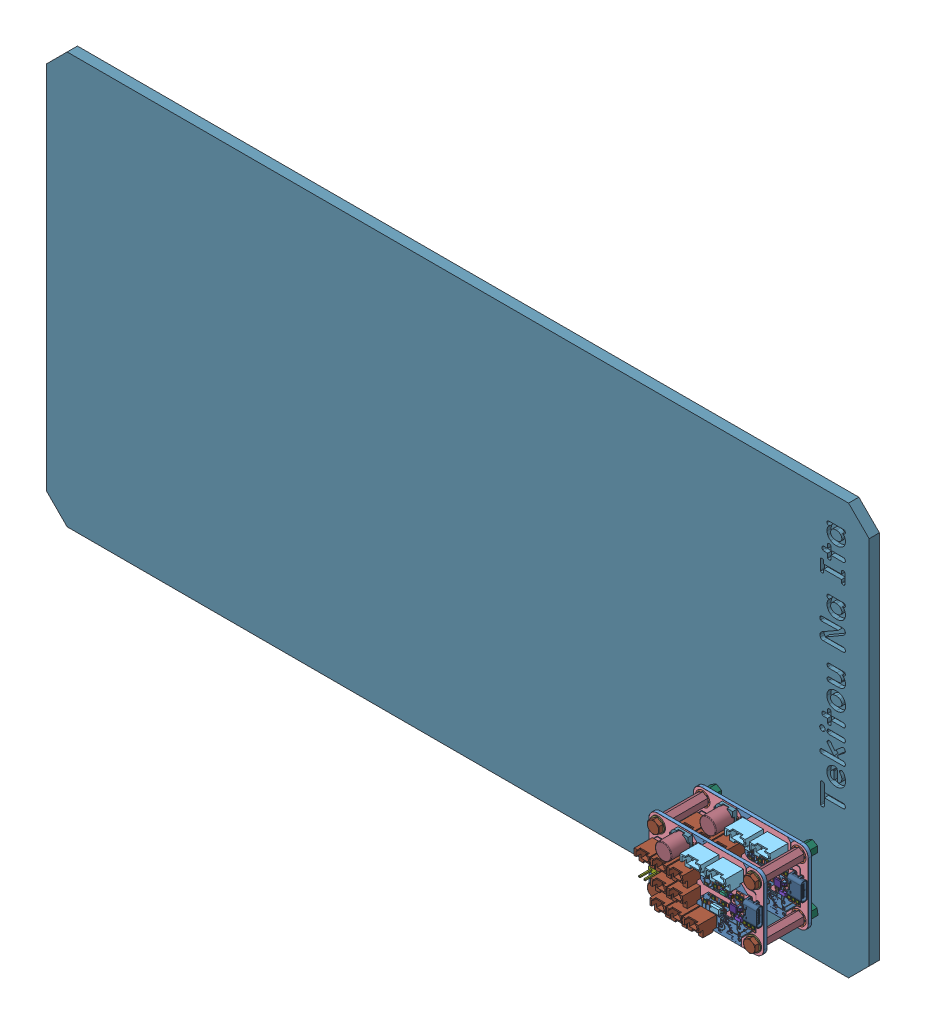
SolidWorks assembly USB_JST-XH_Converter組立サンプル図, configuration ﾃﾞﾌｫﾙﾄ. Lengths in mm.
Overall size (400 200 53.63).
364 component instances, 69 part files, 31 mates.
Components (placement in the parent):
- Board_Geoms_f1fe-1: Board_Geoms_f1fe [ﾃﾞﾌｫﾙﾄ] at (-33.7897 -17.3903 -15.0698) size (55.86 35.85 1.7)
  - Pcb_f1fe-1: Pcb_f1fe [ﾃﾞﾌｫﾙﾄ] at origin size (55.86 35.85 1.6)
  - topPads_f1fe_1-1: topPads_f1fe_1 [ﾃﾞﾌｫﾙﾄ] at (0 0 0.02) size (53.76 33.72 0)
  - topTracks_f1fe-1: topTracks_f1fe [ﾃﾞﾌｫﾙﾄ] at (0 0 0.01) size (44.55 27.82 0)
  - topZones_f1fe-1: topZones_f1fe [ﾃﾞﾌｫﾙﾄ] at (0 0 0.01) size (55.73 35.75 0)
  - botPads_f1fe-1: botPads_f1fe [ﾃﾞﾌｫﾙﾄ] at (0 0 -1.62) size (53.76 33.72 0)
  - botTracks_f1fe-1: botTracks_f1fe [ﾃﾞﾌｫﾙﾄ] at (0 0 -1.61) size (22.1 13.27 0)
  - botZones_f1fe-1: botZones_f1fe [ﾃﾞﾌｫﾙﾄ] at (0 0 -1.61) size (55.76 35.75 0)
  - bottopSilks_f115-1: bottopSilks_f115 [ﾃﾞﾌｫﾙﾄ] at origin size (54.02 34.57 0.01)
  - botSilks_30d3-1: botSilks_30d3 [ﾃﾞﾌｫﾙﾄ] at (0 0 -1.67) size (46.62 31.58 0.02)
- Step_Models_f1fe-1: Step_Models_f1fe [ﾃﾞﾌｫﾙﾄ] at (-33.7897 -17.3903 -15.0698) size (53.92 34.35 13.46)
  - Top_f1fe_1-1: Top_f1fe_1 [ﾃﾞﾌｫﾙﾄ] at origin size (53.92 34.35 13.46)
    - USB1_CUI_DEVICES_UJC-HP-3-SMT-TR_639B4C46-1: USB1_CUI_DEVICES_UJC-HP-3-SMT-TR_639B4C46 [ﾃﾞﾌｫﾙﾄ] at (171.8711 -104.4286 1.3) x (0 1 0) z (1 0 0) size (8.95 4.27 6.9)
    - PORT1_B02B-XASK-1_639C336B-1: PORT1_B02B-XASK-1_639C336B [ﾃﾞﾌｫﾙﾄ] at (125.984 -101.854 0) x (1 0 0) z (0 -1 0) size (7.5 12.2 6.4)
    - PORT1_B02B-XASK-1_639C336B-2: PORT1_B02B-XASK-1_639C336B [ﾃﾞﾌｫﾙﾄ] at (133.9611 -101.854 0) x (1 0 0) z (0 -1 0) size (7.5 12.2 6.4)
    - PORT1_B02B-XASK-1_639C336B-3: PORT1_B02B-XASK-1_639C336B [ﾃﾞﾌｫﾙﾄ] at (141.986 -101.854 0) x (1 0 0) z (0 -1 0) size (7.5 12.2 6.4)
    - PORT1_B02B-XASK-1_639C336B-4: PORT1_B02B-XASK-1_639C336B [ﾃﾞﾌｫﾙﾄ] at (133.9711 -110.4186 0) x (1 0 0) z (0 -1 0) size (7.5 12.2 6.4)
    - PORT1_B02B-XASK-1_639C336B-5: PORT1_B02B-XASK-1_639C336B [ﾃﾞﾌｫﾙﾄ] at (141.9611 -110.4486 0) x (1 0 0) z (0 -1 0) size (7.5 12.2 6.4)
    - SW2_SMLE1_639B495B-1: SW2_SMLE1_639B495B [ﾃﾞﾌｫﾙﾄ] at (148.5711 -101.9286 0) x (-1 0 0) z (0 1 0) size (1.6 0.36 0.8)
    - R2_RT1220P-101-M004_639B496B-1: R2_RT1220P-101-M004_639B496B [ﾃﾞﾌｫﾙﾄ] at (149.3711 -96.9286 0) x (1 0 0) z (0 -1 0) size (2 0.5 1.25)
      - RT1220P-101-M-1: RT1220P-101-M [ﾃﾞﾌｫﾙﾄ] at origin size (0.4 0.5 1.25)
      - RT1220P-101-M001-1: RT1220P-101-M001 [ﾃﾞﾌｫﾙﾄ] at origin size (0.4 0.5 1.25)
      - RT1220P-101-M002-1: RT1220P-101-M002 [ﾃﾞﾌｫﾙﾄ] at origin size (1.95 0.45 1.25)
      - RT1220P-101-M003-1: RT1220P-101-M003 [ﾃﾞﾌｫﾙﾄ] at origin size (1.2 0.03 1.25)
    - R2_RT1220P-101-M004_639B496B-2: R2_RT1220P-101-M004_639B496B [ﾃﾞﾌｫﾙﾄ] at (164.0711 -102.6286 0) x (0 1 0) z (1 0 0) size (2 0.5 1.25)
      - RT1220P-101-M-1: RT1220P-101-M [ﾃﾞﾌｫﾙﾄ] at origin size (0.4 0.5 1.25)
      - RT1220P-101-M001-1: RT1220P-101-M001 [ﾃﾞﾌｫﾙﾄ] at origin size (0.4 0.5 1.25)
      - RT1220P-101-M002-1: RT1220P-101-M002 [ﾃﾞﾌｫﾙﾄ] at origin size (1.95 0.45 1.25)
      - RT1220P-101-M003-1: RT1220P-101-M003 [ﾃﾞﾌｫﾙﾄ] at origin size (1.2 0.03 1.25)
    - R2_RT1220P-101-M004_639B496B-3: R2_RT1220P-101-M004_639B496B [ﾃﾞﾌｫﾙﾄ] at (166.0711 -102.6286 0) x (0 1 0) z (1 0 0) size (2 0.5 1.25)
      - RT1220P-101-M-1: RT1220P-101-M [ﾃﾞﾌｫﾙﾄ] at origin size (0.4 0.5 1.25)
      - RT1220P-101-M001-1: RT1220P-101-M001 [ﾃﾞﾌｫﾙﾄ] at origin size (0.4 0.5 1.25)
      - RT1220P-101-M002-1: RT1220P-101-M002 [ﾃﾞﾌｫﾙﾄ] at origin size (1.95 0.45 1.25)
      - RT1220P-101-M003-1: RT1220P-101-M003 [ﾃﾞﾌｫﾙﾄ] at origin size (1.2 0.03 1.25)
    - PORT1_B02B-XASK-1_639C336B-6: PORT1_B02B-XASK-1_639C336B [ﾃﾞﾌｫﾙﾄ] at (133.5711 -118.9286 0) x (1 0 0) z (0 -1 0) size (7.5 12.2 6.4)
    - PORT1_B02B-XASK-1_639C336B-7: PORT1_B02B-XASK-1_639C336B [ﾃﾞﾌｫﾙﾄ] at (141.5711 -118.9286 0) x (1 0 0) z (0 -1 0) size (7.5 12.2 6.4)
    - PORT1_B02B-XASK-1_639C336B-8: PORT1_B02B-XASK-1_639C336B [ﾃﾞﾌｫﾙﾄ] at (149.5711 -118.9286 0) x (1 0 0) z (0 -1 0) size (7.5 12.2 6.4)
    - C1_CAP_GCM21B_MUR003_639B4A01-1: C1_CAP_GCM21B_MUR003_639B4A01 [ﾃﾞﾌｫﾙﾄ] at (161.0711 -103.4286 0) size (2.01 1.24 1.25)
      - CAP_GCM21B_MUR-1: CAP_GCM21B_MUR [ﾃﾞﾌｫﾙﾄ] at origin size (1.09 1.21 1.21)
      - CAP_GCM21B_MUR001-1: CAP_GCM21B_MUR001 [ﾃﾞﾌｫﾙﾄ] at origin size (0.46 1.24 1.25)
      - CAP_GCM21B_MUR002-1: CAP_GCM21B_MUR002 [ﾃﾞﾌｫﾙﾄ] at origin size (0.46 1.24 1.25)
    - C1_CAP_GCM21B_MUR003_639B4A01-2: C1_CAP_GCM21B_MUR003_639B4A01 [ﾃﾞﾌｫﾙﾄ] at (165.5711 -106.9286 0) x (0 -1 0) z (0 0 1) size (2.01 1.24 1.25)
      - CAP_GCM21B_MUR-1: CAP_GCM21B_MUR [ﾃﾞﾌｫﾙﾄ] at origin size (1.09 1.21 1.21)
      - CAP_GCM21B_MUR001-1: CAP_GCM21B_MUR001 [ﾃﾞﾌｫﾙﾄ] at origin size (0.46 1.24 1.25)
      - CAP_GCM21B_MUR002-1: CAP_GCM21B_MUR002 [ﾃﾞﾌｫﾙﾄ] at origin size (0.46 1.24 1.25)
    - R2_RT1220P-101-M004_639B496B-4: R2_RT1220P-101-M004_639B496B [ﾃﾞﾌｫﾙﾄ] at (171.5711 -111.6286 0) x (0 1 0) z (1 0 0) size (2 0.5 1.25)
      - RT1220P-101-M-1: RT1220P-101-M [ﾃﾞﾌｫﾙﾄ] at origin size (0.4 0.5 1.25)
      - RT1220P-101-M001-1: RT1220P-101-M001 [ﾃﾞﾌｫﾙﾄ] at origin size (0.4 0.5 1.25)
      - RT1220P-101-M002-1: RT1220P-101-M002 [ﾃﾞﾌｫﾙﾄ] at origin size (1.95 0.45 1.25)
      - RT1220P-101-M003-1: RT1220P-101-M003 [ﾃﾞﾌｫﾙﾄ] at origin size (1.2 0.03 1.25)
    - R2_RT1220P-101-M004_639B496B-5: R2_RT1220P-101-M004_639B496B [ﾃﾞﾌｫﾙﾄ] at (167.5711 -111.6286 0) x (0 1 0) z (1 0 0) size (2 0.5 1.25)
      - RT1220P-101-M-1: RT1220P-101-M [ﾃﾞﾌｫﾙﾄ] at origin size (0.4 0.5 1.25)
      - RT1220P-101-M001-1: RT1220P-101-M001 [ﾃﾞﾌｫﾙﾄ] at origin size (0.4 0.5 1.25)
      - RT1220P-101-M002-1: RT1220P-101-M002 [ﾃﾞﾌｫﾙﾄ] at origin size (1.95 0.45 1.25)
      - RT1220P-101-M003-1: RT1220P-101-M003 [ﾃﾞﾌｫﾙﾄ] at origin size (1.2 0.03 1.25)
    - R2_RT1220P-101-M004_639B496B-6: R2_RT1220P-101-M004_639B496B [ﾃﾞﾌｫﾙﾄ] at (153.5711 -100.2286 0) x (0 -1 0) z (-1 0 0) size (2 0.5 1.25)
      - RT1220P-101-M-1: RT1220P-101-M [ﾃﾞﾌｫﾙﾄ] at origin size (0.4 0.5 1.25)
      - RT1220P-101-M001-1: RT1220P-101-M001 [ﾃﾞﾌｫﾙﾄ] at origin size (0.4 0.5 1.25)
      - RT1220P-101-M002-1: RT1220P-101-M002 [ﾃﾞﾌｫﾙﾄ] at origin size (1.95 0.45 1.25)
      - RT1220P-101-M003-1: RT1220P-101-M003 [ﾃﾞﾌｫﾙﾄ] at origin size (1.2 0.03 1.25)
    - R2_RT1220P-101-M004_639B496B-7: R2_RT1220P-101-M004_639B496B [ﾃﾞﾌｫﾙﾄ] at (154.8711 -96.7286 0) x (1 0 0) z (0 -1 0) size (2 0.5 1.25)
      - RT1220P-101-M-1: RT1220P-101-M [ﾃﾞﾌｫﾙﾄ] at origin size (0.4 0.5 1.25)
      - RT1220P-101-M001-1: RT1220P-101-M001 [ﾃﾞﾌｫﾙﾄ] at origin size (0.4 0.5 1.25)
      - RT1220P-101-M002-1: RT1220P-101-M002 [ﾃﾞﾌｫﾙﾄ] at origin size (1.95 0.45 1.25)
      - RT1220P-101-M003-1: RT1220P-101-M003 [ﾃﾞﾌｫﾙﾄ] at origin size (1.2 0.03 1.25)
    - R2_RT1220P-101-M004_639B496B-8: R2_RT1220P-101-M004_639B496B [ﾃﾞﾌｫﾙﾄ] at (156.8711 -101.4286 0) x (1 0 0) z (0 -1 0) size (2 0.5 1.25)
      - RT1220P-101-M-1: RT1220P-101-M [ﾃﾞﾌｫﾙﾄ] at origin size (0.4 0.5 1.25)
      - RT1220P-101-M001-1: RT1220P-101-M001 [ﾃﾞﾌｫﾙﾄ] at origin size (0.4 0.5 1.25)
      - RT1220P-101-M002-1: RT1220P-101-M002 [ﾃﾞﾌｫﾙﾄ] at origin size (1.95 0.45 1.25)
      - RT1220P-101-M003-1: RT1220P-101-M003 [ﾃﾞﾌｫﾙﾄ] at origin size (1.2 0.03 1.25)
    - R2_RT1220P-101-M004_639B496B-9: R2_RT1220P-101-M004_639B496B [ﾃﾞﾌｫﾙﾄ] at (153.2711 -103.4286 0) x (-1 0 0) z (0 1 0) size (2 0.5 1.25)
      - RT1220P-101-M-1: RT1220P-101-M [ﾃﾞﾌｫﾙﾄ] at origin size (0.4 0.5 1.25)
      - RT1220P-101-M001-1: RT1220P-101-M001 [ﾃﾞﾌｫﾙﾄ] at origin size (0.4 0.5 1.25)
      - RT1220P-101-M002-1: RT1220P-101-M002 [ﾃﾞﾌｫﾙﾄ] at origin size (1.95 0.45 1.25)
      - RT1220P-101-M003-1: RT1220P-101-M003 [ﾃﾞﾌｫﾙﾄ] at origin size (1.2 0.03 1.25)
    - R2_RT1220P-101-M004_639B496B-10: R2_RT1220P-101-M004_639B496B [ﾃﾞﾌｫﾙﾄ] at (152.2711 -108.9286 0) x (-1 0 0) z (0 1 0) size (2 0.5 1.25)
      - RT1220P-101-M-1: RT1220P-101-M [ﾃﾞﾌｫﾙﾄ] at origin size (0.4 0.5 1.25)
      - RT1220P-101-M001-1: RT1220P-101-M001 [ﾃﾞﾌｫﾙﾄ] at origin size (0.4 0.5 1.25)
      - RT1220P-101-M002-1: RT1220P-101-M002 [ﾃﾞﾌｫﾙﾄ] at origin size (1.95 0.45 1.25)
      - RT1220P-101-M003-1: RT1220P-101-M003 [ﾃﾞﾌｫﾙﾄ] at origin size (1.2 0.03 1.25)
    - R2_RT1220P-101-M004_639B496B-11: R2_RT1220P-101-M004_639B496B [ﾃﾞﾌｫﾙﾄ] at (157.2711 -108.9286 0) x (-1 0 0) z (0 1 0) size (2 0.5 1.25)
      - RT1220P-101-M-1: RT1220P-101-M [ﾃﾞﾌｫﾙﾄ] at origin size (0.4 0.5 1.25)
      - RT1220P-101-M001-1: RT1220P-101-M001 [ﾃﾞﾌｫﾙﾄ] at origin size (0.4 0.5 1.25)
      - RT1220P-101-M002-1: RT1220P-101-M002 [ﾃﾞﾌｫﾙﾄ] at origin size (1.95 0.45 1.25)
      - RT1220P-101-M003-1: RT1220P-101-M003 [ﾃﾞﾌｫﾙﾄ] at origin size (1.2 0.03 1.25)
    - U2_TLP293(E005_639B4A97-1: U2_TLP293(E005_639B4A97 [ﾃﾞﾌｫﾙﾄ] at (154.5711 -111.9286 0) x (0 -1 0) z (-1 0 0) size (2.6 2.3 7)
      - TLP293(E-1: TLP293(E [ﾃﾞﾌｫﾙﾄ] at origin size (0.38 1.35 1.25)
      - TLP293(E001-1: TLP293(E001 [ﾃﾞﾌｫﾙﾄ] at origin size (0.38 1.35 1.25)
      - TLP293(E002-1: TLP293(E002 [ﾃﾞﾌｫﾙﾄ] at origin size (0.38 1.35 1.25)
      - TLP293(E003-1: TLP293(E003 [ﾃﾞﾌｫﾙﾄ] at origin size (2.6 2.2 4.55)
      - TLP293(E004-1: TLP293(E004 [ﾃﾞﾌｫﾙﾄ] at origin size (0.38 1.35 1.25)
    - R2_RT1220P-101-M004_639B496B-12: R2_RT1220P-101-M004_639B496B [ﾃﾞﾌｫﾙﾄ] at (148.2711 -112.4286 0) x (-1 0 0) z (0 1 0) size (2 0.5 1.25)
      - RT1220P-101-M-1: RT1220P-101-M [ﾃﾞﾌｫﾙﾄ] at origin size (0.4 0.5 1.25)
      - RT1220P-101-M001-1: RT1220P-101-M001 [ﾃﾞﾌｫﾙﾄ] at origin size (0.4 0.5 1.25)
      - RT1220P-101-M002-1: RT1220P-101-M002 [ﾃﾞﾌｫﾙﾄ] at origin size (1.95 0.45 1.25)
      - RT1220P-101-M003-1: RT1220P-101-M003 [ﾃﾞﾌｫﾙﾄ] at origin size (1.2 0.03 1.25)
    - R2_RT1220P-101-M004_639B496B-13: R2_RT1220P-101-M004_639B496B [ﾃﾞﾌｫﾙﾄ] at (169.5711 -111.6286 0) x (0 1 0) z (1 0 0) size (2 0.5 1.25)
      - RT1220P-101-M-1: RT1220P-101-M [ﾃﾞﾌｫﾙﾄ] at origin size (0.4 0.5 1.25)
      - RT1220P-101-M001-1: RT1220P-101-M001 [ﾃﾞﾌｫﾙﾄ] at origin size (0.4 0.5 1.25)
      - RT1220P-101-M002-1: RT1220P-101-M002 [ﾃﾞﾌｫﾙﾄ] at origin size (1.95 0.45 1.25)
      - RT1220P-101-M003-1: RT1220P-101-M003 [ﾃﾞﾌｫﾙﾄ] at origin size (1.2 0.03 1.25)
    - JP1_PinHeader_1x02_P254mm_Vertical_639B4B42-1: JP1_PinHeader_1x02_P254mm_Vertical_639B4B42 [ﾃﾞﾌｫﾙﾄ] at (124.3011 -109.9286 0) x (0 1 0) z (0 0 1) size (2.54 5.08 11.54)
    - TR1_S-Mini-ZKN004_639B4B58-1: TR1_S-Mini-ZKN004_639B4B58 [ﾃﾞﾌｫﾙﾄ] at (164.8711 -111.2286 0) size (2.9 2.5 1.15)
      - S-Mini-ZKN-1: S-Mini-ZKN [ﾃﾞﾌｫﾙﾄ] at origin size (2.9 1.5 1.1)
      - S-Mini-ZKN001-1: S-Mini-ZKN001 [ﾃﾞﾌｫﾙﾄ] at origin size (0.4 0.51 0.85)
      - S-Mini-ZKN002-1: S-Mini-ZKN002 [ﾃﾞﾌｫﾙﾄ] at origin size (0.4 0.51 0.85)
      - S-Mini-ZKN003-1: S-Mini-ZKN003 [ﾃﾞﾌｫﾙﾄ] at origin size (0.4 0.51 0.85)
    - D2_1N914BWT004_639B4B74-1: D2_1N914BWT004_639B4B74 [ﾃﾞﾌｫﾙﾄ] at (167.5711 -106.6286 0) x (0 -1 0) z (-1 0 0) size (1.6 0.7 0.8)
      - 1N914BWT-1: 1N914BWT [ﾃﾞﾌｫﾙﾄ] at origin size (1.2 0.7 0.8)
      - 1N914BWT001-1: 1N914BWT001 [ﾃﾞﾌｫﾙﾄ] at origin size (0.02 0.05 0.5)
      - 1N914BWT002-1: 1N914BWT002 [ﾃﾞﾌｫﾙﾄ] at origin size (0.2 0.2 0.3)
      - 1N914BWT003-1: 1N914BWT003 [ﾃﾞﾌｫﾙﾄ] at origin size (0.2 0.2 0.3)
    - D2_1N914BWT004_639B4B74-2: D2_1N914BWT004_639B4B74 [ﾃﾞﾌｫﾙﾄ] at (160.5711 -101.4286 0) x (1 0 0) z (0 -1 0) size (1.6 0.7 0.8)
      - 1N914BWT-1: 1N914BWT [ﾃﾞﾌｫﾙﾄ] at origin size (1.2 0.7 0.8)
      - 1N914BWT001-1: 1N914BWT001 [ﾃﾞﾌｫﾙﾄ] at origin size (0.02 0.05 0.5)
      - 1N914BWT002-1: 1N914BWT002 [ﾃﾞﾌｫﾙﾄ] at origin size (0.2 0.2 0.3)
      - 1N914BWT003-1: 1N914BWT003 [ﾃﾞﾌｫﾙﾄ] at origin size (0.2 0.2 0.3)
    - D2_1N914BWT004_639B4B74-3: D2_1N914BWT004_639B4B74 [ﾃﾞﾌｫﾙﾄ] at (160.5711 -99.9286 0) x (1 0 0) z (0 -1 0) size (1.6 0.7 0.8)
      - 1N914BWT-1: 1N914BWT [ﾃﾞﾌｫﾙﾄ] at origin size (1.2 0.7 0.8)
      - 1N914BWT001-1: 1N914BWT001 [ﾃﾞﾌｫﾙﾄ] at origin size (0.02 0.05 0.5)
      - 1N914BWT002-1: 1N914BWT002 [ﾃﾞﾌｫﾙﾄ] at origin size (0.2 0.2 0.3)
      - 1N914BWT003-1: 1N914BWT003 [ﾃﾞﾌｫﾙﾄ] at origin size (0.2 0.2 0.3)
    - D2_1N914BWT004_639B4B74-4: D2_1N914BWT004_639B4B74 [ﾃﾞﾌｫﾙﾄ] at (160.5711 -98.4286 0) x (1 0 0) z (0 -1 0) size (1.6 0.7 0.8)
      - 1N914BWT-1: 1N914BWT [ﾃﾞﾌｫﾙﾄ] at origin size (1.2 0.7 0.8)
      - 1N914BWT001-1: 1N914BWT001 [ﾃﾞﾌｫﾙﾄ] at origin size (0.02 0.05 0.5)
      - 1N914BWT002-1: 1N914BWT002 [ﾃﾞﾌｫﾙﾄ] at origin size (0.2 0.2 0.3)
      - 1N914BWT003-1: 1N914BWT003 [ﾃﾞﾌｫﾙﾄ] at origin size (0.2 0.2 0.3)
    - COMP1_part007_639B4BA4-1: COMP1_part007_639B4BA4 [ﾃﾞﾌｫﾙﾄ] at (156.6711 -98.9286 0) x (-1 0 0) z (0 0 1) size (2.39 2.27 1.1)
      - part-1: part [ﾃﾞﾌｫﾙﾄ] at origin size (0.07 0.07 0)
      - part001-1: part001 [ﾃﾞﾌｫﾙﾄ] at origin size (1.35 2.27 1)
      - part002-1: part002 [ﾃﾞﾌｫﾙﾄ] at origin size (0.52 0.41 0.73)
      - part003-1: part003 [ﾃﾞﾌｫﾙﾄ] at origin size (0.52 0.41 0.73)
      - part004-1: part004 [ﾃﾞﾌｫﾙﾄ] at origin size (0.52 0.41 0.73)
      - part005-1: part005 [ﾃﾞﾌｫﾙﾄ] at origin size (0.52 0.41 0.73)
      - part006-1: part006 [ﾃﾞﾌｫﾙﾄ] at origin size (0.52 0.41 0.73)
    - SW2_SMLE1_639B495B-2: SW2_SMLE1_639B495B [ﾃﾞﾌｫﾙﾄ] at (148.5711 -104.8 0) x (-1 0 0) z (0 1 0) size (1.6 0.36 0.8)
    - R2_RT1220P-101-M004_639B496B-14: R2_RT1220P-101-M004_639B496B [ﾃﾞﾌｫﾙﾄ] at (149.3711 -98.9286 0) x (1 0 0) z (0 -1 0) size (2 0.5 1.25)
      - RT1220P-101-M-1: RT1220P-101-M [ﾃﾞﾌｫﾙﾄ] at origin size (0.4 0.5 1.25)
      - RT1220P-101-M001-1: RT1220P-101-M001 [ﾃﾞﾌｫﾙﾄ] at origin size (0.4 0.5 1.25)
      - RT1220P-101-M002-1: RT1220P-101-M002 [ﾃﾞﾌｫﾙﾄ] at origin size (1.95 0.45 1.25)
      - RT1220P-101-M003-1: RT1220P-101-M003 [ﾃﾞﾌｫﾙﾄ] at origin size (1.2 0.03 1.25)
    - POWER_B03B-XASK-1_639B4BD1-1: POWER_B03B-XASK-1_639B4BD1 [ﾃﾞﾌｫﾙﾄ] at (149.5711 -92.9286 0) x (1 0 0) z (0 -1 0) size (10 12.2 6.4)
    - POWER_B03B-XASK-1_639B4BD1-2: POWER_B03B-XASK-1_639B4BD1 [ﾃﾞﾌｫﾙﾄ] at (161.5711 -92.9286 0) x (1 0 0) z (0 -1 0) size (10 12.2 6.4)
    - FET1_ASSEMBLY_639B4C0B-1: FET1_ASSEMBLY_639B4C0B [ﾃﾞﾌｫﾙﾄ] at (157.3711 -104.1286 0) x (0 -1 0) z (0 0 1) size (2.4 2.92 1.2)
      - Body-1: Body [ﾃﾞﾌｫﾙﾄ] at origin size (1.33 2.92 1.15)
      - PinsArrayL002-1: PinsArrayL002 [ﾃﾞﾌｫﾙﾄ] at origin size (0.54 2.39 0.66)
        - PinsArrayL-1: PinsArrayL [ﾃﾞﾌｫﾙﾄ] at origin size (0.54 0.49 0.66)
        - PinsArrayL001-1: PinsArrayL001 [ﾃﾞﾌｫﾙﾄ] at origin size (0.54 0.49 0.66)
      - FilletPinR-1: FilletPinR [ﾃﾞﾌｫﾙﾄ] at origin size (0.54 0.49 0.66)
    - C3_GQM1885C1H8R2CB01J003_639B4C15-1: C3_GQM1885C1H8R2CB01J003_639B4C15 [ﾃﾞﾌｫﾙﾄ] at (161.5711 -110.7786 0) x (-1 0 0) z (0 0 1) size (1.6 0.9 0.8)
      - GQM1885C1H8R2CB01J-1: GQM1885C1H8R2CB01J [ﾃﾞﾌｫﾙﾄ] at origin size (0.35 0.9 0.8)
      - GQM1885C1H8R2CB01J001-1: GQM1885C1H8R2CB01J001 [ﾃﾞﾌｫﾙﾄ] at origin size (0.35 0.9 0.8)
      - GQM1885C1H8R2CB01J002-1: GQM1885C1H8R2CB01J002 [ﾃﾞﾌｫﾙﾄ] at origin size (0.9 0.87 0.77)
    - C4_U2-P_NCH(繝輔ぅ繝ｬ繝・ヨ蠕・004_639B4C24-1: C4_U2-P_NCH(繝輔ぅ繝ｬ繝・ヨ蠕・004_639B4C24 [ﾃﾞﾌｫﾙﾄ] at (137.5711 -91.9286 0) size (8.89 8.31 10.06)
      - U2-P_NCH(繝輔ぅ繝ｬ繝・ヨ蠕・-1: U2-P_NCH(繝輔ぅ繝ｬ繝・ヨ蠕・ [ﾃﾞﾌｫﾙﾄ] at origin size (7.89 7.89 9.01)
      - U2-P_NCH(繝輔ぅ繝ｬ繝・ヨ蠕・001-1: U2-P_NCH(繝輔ぅ繝ｬ繝・ヨ蠕・001 [ﾃﾞﾌｫﾙﾄ] at origin size (8.31 8.31 2)
      - U2-P_NCH(繝輔ぅ繝ｬ繝・ヨ蠕・002-1: U2-P_NCH(繝輔ぅ繝ｬ繝・ヨ蠕・002 [ﾃﾞﾌｫﾙﾄ] at origin size (3.3 0.81 0.25)
      - U2-P_NCH(繝輔ぅ繝ｬ繝・ヨ蠕・003-1: U2-P_NCH(繝輔ぅ繝ｬ繝・ヨ蠕・003 [ﾃﾞﾌｫﾙﾄ] at origin size (3.3 0.81 0.25)
    - U1_WSON10B_Assy_new_ver014_639B4C30-1: U1_WSON10B_Assy_new_ver014_639B4C30 [ﾃﾞﾌｫﾙﾄ] at (162.0711 -108.4286 0) x (0 1 0) z (0 0 1) size (3 3 0.75)
      - WSON10B_Assy_new_ver2-1: WSON10B_Assy_new_ver2 [ﾃﾞﾌｫﾙﾄ] at origin size (3 3 0.7)
      - WSON10B_Assy_new_ver003-1: WSON10B_Assy_new_ver003 [ﾃﾞﾌｫﾙﾄ] at origin size (3 1.65 0.1)
      - WSON10B_Assy_new_ver004-1: WSON10B_Assy_new_ver004 [ﾃﾞﾌｫﾙﾄ] at origin size (0.24 0.4 0.2)
      - WSON10B_Assy_new_ver005-1: WSON10B_Assy_new_ver005 [ﾃﾞﾌｫﾙﾄ] at origin size (0.24 0.4 0.2)
      - WSON10B_Assy_new_ver006-1: WSON10B_Assy_new_ver006 [ﾃﾞﾌｫﾙﾄ] at origin size (0.24 0.4 0.2)
      - WSON10B_Assy_new_ver007-1: WSON10B_Assy_new_ver007 [ﾃﾞﾌｫﾙﾄ] at origin size (0.24 0.4 0.2)
      - WSON10B_Assy_new_ver008-1: WSON10B_Assy_new_ver008 [ﾃﾞﾌｫﾙﾄ] at origin size (0.24 0.4 0.2)
      - WSON10B_Assy_new_ver009-1: WSON10B_Assy_new_ver009 [ﾃﾞﾌｫﾙﾄ] at origin size (0.24 0.4 0.2)
      - WSON10B_Assy_new_ver010-1: WSON10B_Assy_new_ver010 [ﾃﾞﾌｫﾙﾄ] at origin size (0.24 0.4 0.2)
      - WSON10B_Assy_new_ver011-1: WSON10B_Assy_new_ver011 [ﾃﾞﾌｫﾙﾄ] at origin size (0.24 0.4 0.2)
      - WSON10B_Assy_new_ver012-1: WSON10B_Assy_new_ver012 [ﾃﾞﾌｫﾙﾄ] at origin size (0.24 0.4 0.2)
      - WSON10B_Assy_new_ver013-1: WSON10B_Assy_new_ver013 [ﾃﾞﾌｫﾙﾄ] at origin size (0.24 0.4 0.2)
- USB_JST-XH_Converter組立図-1: USB_JST-XH_Converter組立図 [ﾃﾞﾌｫﾙﾄ] at (-33.7897 -17.3903 6.5602) size (55.86 35.85 14.61)
  - Board_Geoms_f1fe-1: Board_Geoms_f1fe [ﾃﾞﾌｫﾙﾄ] at origin size (55.86 35.85 1.7)
    - Pcb_f1fe-1: Pcb_f1fe [ﾃﾞﾌｫﾙﾄ] at origin size (55.86 35.85 1.6)
    - topPads_f1fe_1-1: topPads_f1fe_1 [ﾃﾞﾌｫﾙﾄ] at (0 0 0.02) size (53.76 33.72 0)
    - topTracks_f1fe-1: topTracks_f1fe [ﾃﾞﾌｫﾙﾄ] at (0 0 0.01) size (44.55 27.82 0)
    - topZones_f1fe-1: topZones_f1fe [ﾃﾞﾌｫﾙﾄ] at (0 0 0.01) size (55.73 35.75 0)
    - botPads_f1fe-1: botPads_f1fe [ﾃﾞﾌｫﾙﾄ] at (0 0 -1.62) size (53.76 33.72 0)
    - botTracks_f1fe-1: botTracks_f1fe [ﾃﾞﾌｫﾙﾄ] at (0 0 -1.61) size (22.1 13.27 0)
    - botZones_f1fe-1: botZones_f1fe [ﾃﾞﾌｫﾙﾄ] at (0 0 -1.61) size (55.76 35.75 0)
    - bottopSilks_f115-1: bottopSilks_f115 [ﾃﾞﾌｫﾙﾄ] at origin size (54.02 34.57 0.01)
    - botSilks_30d3-1: botSilks_30d3 [ﾃﾞﾌｫﾙﾄ] at (0 0 -1.67) size (46.62 31.58 0.02)
  - Step_Models_f1fe-1: Step_Models_f1fe [ﾃﾞﾌｫﾙﾄ] at origin size (53.92 34.35 13.46)
    - Top_f1fe_1-1: Top_f1fe_1 [ﾃﾞﾌｫﾙﾄ] at origin size (53.92 34.35 13.46)
      - USB1_CUI_DEVICES_UJC-HP-3-SMT-TR_639B4C46-1: USB1_CUI_DEVICES_UJC-HP-3-SMT-TR_639B4C46 [ﾃﾞﾌｫﾙﾄ] at (171.8711 -104.4286 1.3) x (0 1 0) z (1 0 0) size (8.95 4.27 6.9)
      - PORT1_B02B-XASK-1_639C336B-1: PORT1_B02B-XASK-1_639C336B [ﾃﾞﾌｫﾙﾄ] at (125.984 -101.854 0) x (1 0 0) z (0 -1 0) size (7.5 12.2 6.4)
      - PORT1_B02B-XASK-1_639C336B-2: PORT1_B02B-XASK-1_639C336B [ﾃﾞﾌｫﾙﾄ] at (133.9611 -101.854 0) x (1 0 0) z (0 -1 0) size (7.5 12.2 6.4)
      - PORT1_B02B-XASK-1_639C336B-3: PORT1_B02B-XASK-1_639C336B [ﾃﾞﾌｫﾙﾄ] at (141.986 -101.854 0) x (1 0 0) z (0 -1 0) size (7.5 12.2 6.4)
      - PORT1_B02B-XASK-1_639C336B-4: PORT1_B02B-XASK-1_639C336B [ﾃﾞﾌｫﾙﾄ] at (133.9711 -110.4186 0) x (1 0 0) z (0 -1 0) size (7.5 12.2 6.4)
      - PORT1_B02B-XASK-1_639C336B-5: PORT1_B02B-XASK-1_639C336B [ﾃﾞﾌｫﾙﾄ] at (141.9611 -110.4486 0) x (1 0 0) z (0 -1 0) size (7.5 12.2 6.4)
      - SW2_SMLE1_639B495B-1: SW2_SMLE1_639B495B [ﾃﾞﾌｫﾙﾄ] at (148.5711 -101.9286 0) x (-1 0 0) z (0 1 0) size (1.6 0.36 0.8)
      - R2_RT1220P-101-M004_639B496B-1: R2_RT1220P-101-M004_639B496B [ﾃﾞﾌｫﾙﾄ] at (149.3711 -96.9286 0) x (1 0 0) z (0 -1 0) size (2 0.5 1.25)
        - RT1220P-101-M-1: RT1220P-101-M [ﾃﾞﾌｫﾙﾄ] at origin size (0.4 0.5 1.25)
        - RT1220P-101-M001-1: RT1220P-101-M001 [ﾃﾞﾌｫﾙﾄ] at origin size (0.4 0.5 1.25)
        - RT1220P-101-M002-1: RT1220P-101-M002 [ﾃﾞﾌｫﾙﾄ] at origin size (1.95 0.45 1.25)
        - RT1220P-101-M003-1: RT1220P-101-M003 [ﾃﾞﾌｫﾙﾄ] at origin size (1.2 0.03 1.25)
      - R2_RT1220P-101-M004_639B496B-2: R2_RT1220P-101-M004_639B496B [ﾃﾞﾌｫﾙﾄ] at (164.0711 -102.6286 0) x (0 1 0) z (1 0 0) size (2 0.5 1.25)
        - RT1220P-101-M-1: RT1220P-101-M [ﾃﾞﾌｫﾙﾄ] at origin size (0.4 0.5 1.25)
        - RT1220P-101-M001-1: RT1220P-101-M001 [ﾃﾞﾌｫﾙﾄ] at origin size (0.4 0.5 1.25)
        - RT1220P-101-M002-1: RT1220P-101-M002 [ﾃﾞﾌｫﾙﾄ] at origin size (1.95 0.45 1.25)
        - RT1220P-101-M003-1: RT1220P-101-M003 [ﾃﾞﾌｫﾙﾄ] at origin size (1.2 0.03 1.25)
      - R2_RT1220P-101-M004_639B496B-3: R2_RT1220P-101-M004_639B496B [ﾃﾞﾌｫﾙﾄ] at (166.0711 -102.6286 0) x (0 1 0) z (1 0 0) size (2 0.5 1.25)
        - RT1220P-101-M-1: RT1220P-101-M [ﾃﾞﾌｫﾙﾄ] at origin size (0.4 0.5 1.25)
        - RT1220P-101-M001-1: RT1220P-101-M001 [ﾃﾞﾌｫﾙﾄ] at origin size (0.4 0.5 1.25)
        - RT1220P-101-M002-1: RT1220P-101-M002 [ﾃﾞﾌｫﾙﾄ] at origin size (1.95 0.45 1.25)
        - RT1220P-101-M003-1: RT1220P-101-M003 [ﾃﾞﾌｫﾙﾄ] at origin size (1.2 0.03 1.25)
      - PORT1_B02B-XASK-1_639C336B-6: PORT1_B02B-XASK-1_639C336B [ﾃﾞﾌｫﾙﾄ] at (133.5711 -118.9286 0) x (1 0 0) z (0 -1 0) size (7.5 12.2 6.4)
      - PORT1_B02B-XASK-1_639C336B-7: PORT1_B02B-XASK-1_639C336B [ﾃﾞﾌｫﾙﾄ] at (141.5711 -118.9286 0) x (1 0 0) z (0 -1 0) size (7.5 12.2 6.4)
      - PORT1_B02B-XASK-1_639C336B-8: PORT1_B02B-XASK-1_639C336B [ﾃﾞﾌｫﾙﾄ] at (149.5711 -118.9286 0) x (1 0 0) z (0 -1 0) size (7.5 12.2 6.4)
      - C1_CAP_GCM21B_MUR003_639B4A01-1: C1_CAP_GCM21B_MUR003_639B4A01 [ﾃﾞﾌｫﾙﾄ] at (161.0711 -103.4286 0) size (2.01 1.24 1.25)
        - CAP_GCM21B_MUR-1: CAP_GCM21B_MUR [ﾃﾞﾌｫﾙﾄ] at origin size (1.09 1.21 1.21)
        - CAP_GCM21B_MUR001-1: CAP_GCM21B_MUR001 [ﾃﾞﾌｫﾙﾄ] at origin size (0.46 1.24 1.25)
        - CAP_GCM21B_MUR002-1: CAP_GCM21B_MUR002 [ﾃﾞﾌｫﾙﾄ] at origin size (0.46 1.24 1.25)
      - C1_CAP_GCM21B_MUR003_639B4A01-2: C1_CAP_GCM21B_MUR003_639B4A01 [ﾃﾞﾌｫﾙﾄ] at (165.5711 -106.9286 0) x (0 -1 0) z (0 0 1) size (2.01 1.24 1.25)
        - CAP_GCM21B_MUR-1: CAP_GCM21B_MUR [ﾃﾞﾌｫﾙﾄ] at origin size (1.09 1.21 1.21)
        - CAP_GCM21B_MUR001-1: CAP_GCM21B_MUR001 [ﾃﾞﾌｫﾙﾄ] at origin size (0.46 1.24 1.25)
        - CAP_GCM21B_MUR002-1: CAP_GCM21B_MUR002 [ﾃﾞﾌｫﾙﾄ] at origin size (0.46 1.24 1.25)
      - R2_RT1220P-101-M004_639B496B-4: R2_RT1220P-101-M004_639B496B [ﾃﾞﾌｫﾙﾄ] at (171.5711 -111.6286 0) x (0 1 0) z (1 0 0) size (2 0.5 1.25)
        - RT1220P-101-M-1: RT1220P-101-M [ﾃﾞﾌｫﾙﾄ] at origin size (0.4 0.5 1.25)
        - RT1220P-101-M001-1: RT1220P-101-M001 [ﾃﾞﾌｫﾙﾄ] at origin size (0.4 0.5 1.25)
        - RT1220P-101-M002-1: RT1220P-101-M002 [ﾃﾞﾌｫﾙﾄ] at origin size (1.95 0.45 1.25)
        - RT1220P-101-M003-1: RT1220P-101-M003 [ﾃﾞﾌｫﾙﾄ] at origin size (1.2 0.03 1.25)
      - R2_RT1220P-101-M004_639B496B-5: R2_RT1220P-101-M004_639B496B [ﾃﾞﾌｫﾙﾄ] at (167.5711 -111.6286 0) x (0 1 0) z (1 0 0) size (2 0.5 1.25)
        - RT1220P-101-M-1: RT1220P-101-M [ﾃﾞﾌｫﾙﾄ] at origin size (0.4 0.5 1.25)
        - RT1220P-101-M001-1: RT1220P-101-M001 [ﾃﾞﾌｫﾙﾄ] at origin size (0.4 0.5 1.25)
        - RT1220P-101-M002-1: RT1220P-101-M002 [ﾃﾞﾌｫﾙﾄ] at origin size (1.95 0.45 1.25)
        - RT1220P-101-M003-1: RT1220P-101-M003 [ﾃﾞﾌｫﾙﾄ] at origin size (1.2 0.03 1.25)
      - R2_RT1220P-101-M004_639B496B-6: R2_RT1220P-101-M004_639B496B [ﾃﾞﾌｫﾙﾄ] at (153.5711 -100.2286 0) x (0 -1 0) z (-1 0 0) size (2 0.5 1.25)
        - RT1220P-101-M-1: RT1220P-101-M [ﾃﾞﾌｫﾙﾄ] at origin size (0.4 0.5 1.25)
        - RT1220P-101-M001-1: RT1220P-101-M001 [ﾃﾞﾌｫﾙﾄ] at origin size (0.4 0.5 1.25)
        - RT1220P-101-M002-1: RT1220P-101-M002 [ﾃﾞﾌｫﾙﾄ] at origin size (1.95 0.45 1.25)
        - RT1220P-101-M003-1: RT1220P-101-M003 [ﾃﾞﾌｫﾙﾄ] at origin size (1.2 0.03 1.25)
      - R2_RT1220P-101-M004_639B496B-7: R2_RT1220P-101-M004_639B496B [ﾃﾞﾌｫﾙﾄ] at (154.8711 -96.7286 0) x (1 0 0) z (0 -1 0) size (2 0.5 1.25)
        - RT1220P-101-M-1: RT1220P-101-M [ﾃﾞﾌｫﾙﾄ] at origin size (0.4 0.5 1.25)
        - RT1220P-101-M001-1: RT1220P-101-M001 [ﾃﾞﾌｫﾙﾄ] at origin size (0.4 0.5 1.25)
